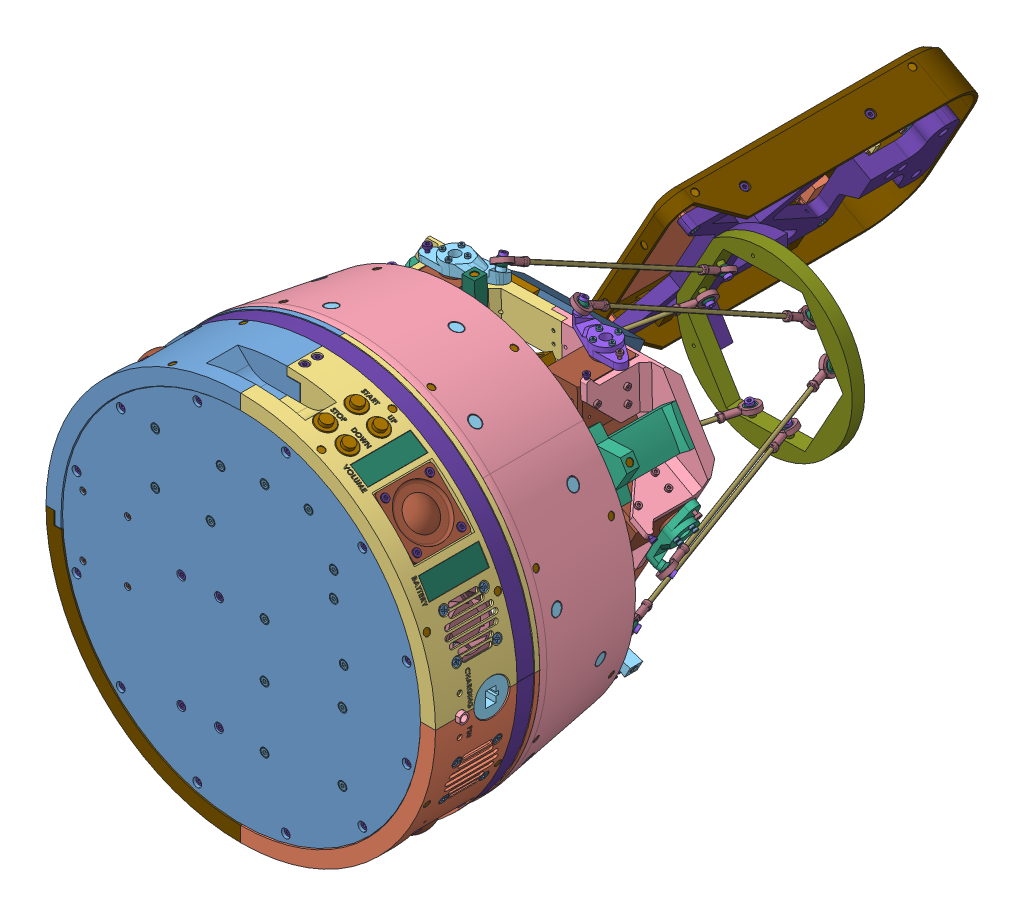
SolidWorks assembly robot xavier, configuration Défaut. Lengths in mm. (continued)
Components (placement in the parent): (continued)
- base-1: base [Défaut] at (-67.3784 29.2661 438.4062) size (438.41 438.41 173) (continued)
  - M3x12mm plastic-7: M3x12mm plastic [Défaut] at (-130.5258 63.5682 511.18) x (-0.383049 0.923728 0) z (0 0 -1) size (5.5 5.5 14.3)
  - M3x12mm plastic-8: M3x12mm plastic [Défaut] at (-130.5258 -42.0524 511.18) x (-0.924031 0.382318 0) z (0 0 -1) size (5.5 5.5 14.3)
  - magnet 5x1.6-2: magnet 5x1.6 [Défaut] at (-144.384 69.3085 585.18) x (-0.146447 -0.353553 0.92388) z (-0.92388 0.382683 0) size (5 5 1.6)
  - magnet 5x1.6-3: magnet 5x1.6 [Défaut] at (-61.581 152.1115 585.18) x (-0.353553 -0.146447 0.92388) z (-0.382683 0.92388 0) size (5 5 1.6)
  - magnet 5x1.6-4: magnet 5x1.6 [Défaut] at (55.5202 152.1115 585.18) x (-0.353553 0.146447 0.92388) z (0.382683 0.92388 0) size (5 5 1.6)
  - magnet 5x1.6-5: magnet 5x1.6 [Défaut] at (138.3232 69.3085 585.18) x (-0.146447 0.353553 0.92388) z (0.92388 0.382683 0) size (5 5 1.6)
  - magnet 5x1.6-6: magnet 5x1.6 [Défaut] at (138.3232 -47.7926 585.18) x (0.146447 0.353553 0.92388) z (0.92388 -0.382683 0) size (5 5 1.6)
  - magnet 5x1.6-7: magnet 5x1.6 [Défaut] at (55.5202 -130.5956 585.18) x (0.353553 0.146447 0.92388) z (0.382683 -0.92388 0) size (5 5 1.6)
  - magnet 5x1.6-8: magnet 5x1.6 [Défaut] at (-61.581 -130.5956 585.18) x (0.353553 -0.146447 0.92388) z (-0.382683 -0.92388 0) size (5 5 1.6)
  - magnet 5x1.6-10: magnet 5x1.6 [Défaut] at (-133.1214 -43.1275 427.3698) x (-0.137009 0.642728 -0.753744) z (-0.912505 -0.377972 -0.156434) size (5 5 1.6)
  - magnet 5x1.6-11: magnet 5x1.6 [Défaut] at (-133.1214 64.6434 427.3698) x (0.357597 0.551357 -0.753744) z (-0.912505 0.377972 -0.156434) size (5 5 1.6)
  - magnet 5x1.6-12: magnet 5x1.6 [Défaut] at (-56.9159 140.849 427.3698) x (0.642728 0.137009 -0.753744) z (-0.377972 0.912505 -0.156434) size (5 5 1.6)
  - magnet 5x1.6-13: magnet 5x1.6 [Défaut] at (50.8551 140.849 427.3698) x (0.551357 -0.357597 -0.753744) z (0.377972 0.912505 -0.156434) size (5 5 1.6)
  - magnet 5x1.6-14: magnet 5x1.6 [Défaut] at (127.0606 64.6434 427.3698) x (0.137009 -0.642728 -0.753744) z (0.912505 0.377972 -0.156434) size (5 5 1.6)
  - magnet 5x1.6-15: magnet 5x1.6 [Défaut] at (127.0606 -43.1275 427.3698) x (-0.357597 -0.551357 -0.753744) z (0.912505 -0.377972 -0.156434) size (5 5 1.6)
  - magnet 5x1.6-16: magnet 5x1.6 [Défaut] at (50.8551 -119.3331 427.3698) x (-0.642728 -0.137009 -0.753744) z (0.377972 -0.912505 -0.156434) size (5 5 1.6)
  - magnet 5x1.6-18: magnet 5x1.6 [Défaut] at (-143.3897 -47.3808 497.5426) x (-0.137009 0.642728 -0.753744) z (-0.912505 -0.377972 -0.156434) size (5 5 1.6)
  - magnet 5x1.6-19: magnet 5x1.6 [Défaut] at (-143.3897 68.8967 497.5426) x (0.357597 0.551357 -0.753744) z (-0.912505 0.377972 -0.156434) size (5 5 1.6)
  - magnet 5x1.6-20: magnet 5x1.6 [Défaut] at (-61.1691 151.1172 497.5426) x (0.642728 0.137009 -0.753744) z (-0.377972 0.912505 -0.156434) size (5 5 1.6)
  - magnet 5x1.6-21: magnet 5x1.6 [Défaut] at (55.1083 151.1172 497.5426) x (0.551357 -0.357597 -0.753744) z (0.377972 0.912505 -0.156434) size (5 5 1.6)
  - magnet 5x1.6-22: magnet 5x1.6 [Défaut] at (137.3289 68.8967 497.5426) x (0.137009 -0.642728 -0.753744) z (0.912505 0.377972 -0.156434) size (5 5 1.6)
  - magnet 5x1.6-23: magnet 5x1.6 [Défaut] at (137.3289 -47.3808 497.5426) x (-0.357597 -0.551357 -0.753744) z (0.912505 -0.377972 -0.156434) size (5 5 1.6)
  - magnet 5x1.6-24: magnet 5x1.6 [Défaut] at (55.1083 -129.6014 497.5426) x (-0.642728 -0.137009 -0.753744) z (0.377972 -0.912505 -0.156434) size (5 5 1.6)
  - magnet 5x1.6-26: magnet 5x1.6 [Défaut] at (-144.384 69.3085 528.68) x (-0.146447 -0.353553 0.92388) z (-0.92388 0.382683 0) size (5 5 1.6)
  - magnet 5x1.6-27: magnet 5x1.6 [Défaut] at (-61.581 152.1115 528.68) x (-0.353553 -0.146447 0.92388) z (-0.382683 0.92388 0) size (5 5 1.6)
  - magnet 5x1.6-28: magnet 5x1.6 [Défaut] at (55.5202 152.1115 528.68) x (-0.353553 0.146447 0.92388) z (0.382683 0.92388 0) size (5 5 1.6)
  - magnet 5x1.6-29: magnet 5x1.6 [Défaut] at (138.3232 69.3085 528.68) x (-0.146447 0.353553 0.92388) z (0.92388 0.382683 0) size (5 5 1.6)
  - magnet 5x1.6-30: magnet 5x1.6 [Défaut] at (138.3232 -47.7926 528.68) x (0.146447 0.353553 0.92388) z (0.92388 -0.382683 0) size (5 5 1.6)
  - magnet 5x1.6-31: magnet 5x1.6 [Défaut] at (55.5202 -130.5956 528.68) x (0.353553 0.146447 0.92388) z (0.382683 -0.92388 0) size (5 5 1.6)
  - magnet 5x1.6-32: magnet 5x1.6 [Défaut] at (-61.581 -130.5956 528.68) x (0.353553 -0.146447 0.92388) z (-0.382683 -0.92388 0) size (5 5 1.6)
- torso bottom xavier-1: torso bottom xavier [Défaut] at (-346.4088 28.5468 798.7391) x (0 0 -1) z (1 0 0) size (138.9 286.86 276.63) (flexible)
  - base gear-1: base gear [Défaut] at (-29.7845 -73.604 101.0471) size (13.91 276 276)
    - base gear 1-1: base gear 1 [Défaut] at (-37.0626 85.0813 174.9529) size (10 121.52 174.95)
    - base gear 2-1: base gear 2 [Défaut] at (-37.0626 85.0813 174.9529) size (10 174.95 121.52)
    - base gear 3-1: base gear 3 [Défaut] at (-37.0626 85.0813 174.9529) size (10 121.52 174.95)
    - base gear 4-1: base gear 4 [Défaut] at (-37.0626 85.0813 174.9529) size (13.91 174.95 121.52)
    - M3x6mm plastic-1: M3x6mm plastic [Défaut] at (-36.0626 58.0825 44.722) x (0 0 -1) z (1 0 0) size (5.5 5.5 8.3)
    - M3x6mm plastic-2: M3x6mm plastic [Défaut] at (-36.0626 215.3121 147.9541) x (0 0 -1) z (1 0 0) size (5.5 5.5 8.3)
    - M3x6mm plastic-3: M3x6mm plastic [Défaut] at (-36.0626 112.08 305.1837) x (0 0 -1) z (1 0 0) size (5.5 5.5 8.3)
    - M3x6mm plastic-4: M3x6mm plastic [Défaut] at (-36.0626 -45.1495 201.9516) x (0 0 -1) z (1 0 0) size (5.5 5.5 8.3)
  - torso bottom external-1: torso bottom external [Défaut] at (174.2366 -65.8734 317.1586) x (0 0.020761 0.999784) z (-1 0 0) size (250 250 10)
    - torso bottom external 1-1: torso bottom external 1 [Défaut] at (-39.5438 78.1885 220.0837) size (220.08 104.52 10)
    - torso bottom external 2-1: torso bottom external 2 [Défaut] at (-39.5438 78.1885 220.0837) size (165.18 170.3 10)
    - torso bottom external 3-1: torso bottom external 3 [Défaut] at (-39.5438 78.1885 220.0837) size (109.03 217.53 10)
    - M3x6mm plastic-1: M3x6mm plastic [Défaut] at (-119.0039 2.1221 229.0837) x (-1 0 0) z (0 0 -1) size (5.5 5.5 8.3)
    - M3x6mm plastic-2: M3x6mm plastic [Défaut] at (-126.2275 -4.793 229.0837) x (-1 0 0) z (0 0 -1) size (5.5 5.5 8.3)
    - M3x6mm plastic-3: M3x6mm plastic [Défaut] at (66.0616 47.4073 229.0837) x (-1 0 0) z (0 0 -1) size (5.5 5.5 8.3)
    - M3x6mm plastic-4: M3x6mm plastic [Défaut] at (75.6621 44.609 229.0837) x (-1 0 0) z (0 0 -1) size (5.5 5.5 8.3)
    - M3x6mm plastic-5: M3x6mm plastic [Défaut] at (-65.6893 185.0362 229.0837) x (-1 0 0) z (0 0 -1) size (5.5 5.5 8.3)
    - M3x6mm plastic-6: M3x6mm plastic [Défaut] at (-68.0662 194.7496 229.0837) x (-1 0 0) z (0 0 -1) size (5.5 5.5 8.3)
  - torso bottom internal xavier-1: torso bottom internal xavier [Défaut] at (-45.8471 11.4773 276) x (0 -0.855458 0.517872) z (-1 0 0) size (168.5 194.56 65)
  - torso bottom holder-1: torso bottom holder [Défaut] at (-69.831 -106.8794 292.5674) x (0 -0.855458 0.517872) z (0 0.517872 0.855458) size (29.5 23 26.69)
    - torso bottom holder-1: torso bottom holder [Défaut] at (-16.159 -8.0161 32.1209) size (29.5 22 26.69)
    - 605zz-1: 605zz [Défaut] at (5.461 -2.0161 24.075) x (0.190809 0 0.981627) z (-0.981627 0 0.190809) size (14 14 5)
    - M5 washer-1: M5 washer [Défaut] at (0.5529 -2.0161 25.029) x (0.190809 0 0.981627) z (-0.981627 0 0.190809) size (10 10 1.1)
    - M5 washer-2: M5 washer [Défaut] at (6.5408 -2.0161 23.8651) x (0.190809 0 0.981627) z (-0.981627 0 0.190809) size (10 10 1.1)
    - M5x16mm socket-1: M5x16mm socket [Défaut] at (10.0747 -2.0161 23.1782) x (-0.981627 0 0.190809) z (-0.132069 -0.72175 -0.679437) size (21 8.5 8.5)
  - torso bottom holder-2: torso bottom holder [Défaut] at (-69.831 85.0034 370.2162) x (0 0.876219 0.481912) z (0 0.481912 -0.876219) size (29.5 23 26.69)
    - torso bottom holder-1: torso bottom holder [Défaut] at (-16.159 -8.0161 32.1209) size (29.5 22 26.69)
    - 605zz-1: 605zz [Défaut] at (5.461 -2.0161 24.075) x (0.190809 0 0.981627) z (-0.981627 0 0.190809) size (14 14 5)
    - M5 washer-1: M5 washer [Défaut] at (0.5529 -2.0161 25.029) x (0.190809 0 0.981627) z (-0.981627 0 0.190809) size (10 10 1.1)
    - M5 washer-2: M5 washer [Défaut] at (6.5408 -2.0161 23.8651) x (0.190809 0 0.981627) z (-0.981627 0 0.190809) size (10 10 1.1)
    - M5x16mm socket-1: M5x16mm socket [Défaut] at (10.0747 -2.0161 23.1782) x (-0.981627 0 0.190809) z (-0.132069 -0.72175 -0.679437) size (21 8.5 8.5)
  - torso bottom holder-3: torso bottom holder [Défaut] at (-69.831 56.3078 165.2164) x (0 -0.020761 -0.999784) z (0 -0.999784 0.020761) size (29.5 23 26.69)
    - torso bottom holder-1: torso bottom holder [Défaut] at (-16.159 -8.0161 32.1209) size (29.5 22 26.69)
    - 605zz-1: 605zz [Défaut] at (5.461 -2.0161 24.075) x (0.190809 0 0.981627) z (-0.981627 0 0.190809) size (14 14 5)
    - M5 washer-1: M5 washer [Défaut] at (0.5529 -2.0161 25.029) x (0.190809 0 0.981627) z (-0.981627 0 0.190809) size (10 10 1.1)
    - M5 washer-2: M5 washer [Défaut] at (6.5408 -2.0161 23.8651) x (0.190809 0 0.981627) z (-0.981627 0 0.190809) size (10 10 1.1)
    - M5x16mm socket-1: M5x16mm socket [Défaut] at (10.0747 -2.0161 23.1782) x (-0.981627 0 0.190809) z (-0.132069 -0.72175 -0.679437) size (21 8.5 8.5)
  - limit switch bracket-1: limit switch bracket [Défaut] at (-45.8471 11.4773 276) x (0 -0.810958 -0.585105) z (1 0 0) size (34.42 36.22 10)
  - stewart stand-1: stewart stand [Défaut] at (-45.8471 11.4773 276) x (0 0.174686 -0.984624) z (1 0 0) size (47.84 42.37 60)
  - stewart stand-2: stewart stand [Défaut] at (-45.8471 11.4773 276) x (0 0.765367 0.643594) z (1 0 0) size (47.84 42.37 60)
  - stewart stand-3: stewart stand [Défaut] at (-45.8471 11.4773 276) x (0 -0.940053 0.34103) z (1 0 0) size (47.84 42.37 60)
  - limit switch-1: limit switch [Défaut] at (-39.8471 -70.7788 381.8891) x (0 0.810958 0.585105) z (0 0.585105 -0.810958) size (20 16.7 6)
  - slip ring (SNM220A-24)-1: slip ring (SNM220A-24) [Défaut] at (-108.3471 11.4773 276) x (0 -0.517872 -0.855458) z (1 0 0) size (44 44 66.3)
  - Jetson AGX Xavier-1: Jetson AGX Xavier [Défaut] at (-61.5471 20.168 283.5975) x (0 -0.855458 0.517872) z (1 0 0) size (105 105 65.46)
  - gear servo bracket-1: gear servo bracket [Défaut] at (-92.1471 -13.8325 196.3361) x (0 0.855458 -0.517872) z (1 0 0) size (80.9 110.9 63)
    - gear servo bracket-1: gear servo bracket [Défaut] at (-19.6043 81.2564 46.3) size (55 84.8 42)
    - XL430-W250-T-1: XL430-W250-T [Défaut] at (-13.6043 10.5064 84.3) x (0 -1 0) z (0 0 -1) size (28.5 46.5 36)
    - torso bottom gear-1: torso bottom gear [Metric - Spur gear 1.5M 52T 20PA 10FW ---S52N75H50L9N] at (-25.6043 10.5064 35.3) x (0 0 -1) z (0 1 0) size (23 80.9 80.9)
    - M2.5x8mm plastic-1: M2.5x8mm plastic [Défaut] at (-21.6043 -0.7436 73.3) x (1 0 0) z (0 -1 0) size (4.5 4.5 9.9)
    - M2.5x8mm plastic-2: M2.5x8mm plastic [Défaut] at (2.3957 -0.7436 73.3) x (1 0 0) z (0 -1 0) size (4.5 4.5 9.9)
    - M2.5x8mm plastic-3: M2.5x8mm plastic [Défaut] at (-21.6043 -0.7436 61.3) x (1 0 0) z (0 -1 0) size (4.5 4.5 9.9)
    - M2.5x8mm plastic-4: M2.5x8mm plastic [Défaut] at (2.3957 -0.7436 61.3) x (1 0 0) z (0 -1 0) size (4.5 4.5 9.9)
    - M2.5x8mm plastic-5: M2.5x8mm plastic [Défaut] at (-34.1043 2.5064 61.3) x (0 0 1) z (-1 0 0) size (4.5 4.5 9.9)
    - M2.5x8mm plastic-6: M2.5x8mm plastic [Défaut] at (-34.1043 18.5064 61.3) x (0 0 1) z (-1 0 0) size (4.5 4.5 9.9)
    - M2x12mm socket-1: M2x12mm socket [Défaut] at (-25.6043 18.5064 51.3) x (-0.923728 -0.383049 0) z (0 0 -1) size (3.8 3.8 13.6)
    - M2x12mm socket-2: M2x12mm socket [Défaut] at (-33.6043 10.5064 51.3) x (1 0 0) z (0 0 -1) size (3.8 3.8 13.6)
    - M2x12mm socket-3: M2x12mm socket [Défaut] at (-17.6043 10.5064 51.3) x (-0.923728 -0.383049 0) z (0 0 -1) size (3.8 3.8 13.6)
    - M2x12mm socket-4: M2x12mm socket [Défaut] at (-25.6043 2.5064 51.3) x (1 0 0) z (0 0 -1) size (3.8 3.8 13.6)
  - torso bottom magnet bracket-1: torso bottom magnet bracket [Défaut] at (-45.8471 11.4773 276) x (0 0.999784 -0.020761) z (1 0 0) size (36.32 10 10)
  - M3x12mm plastic-15: M3x12mm plastic [Défaut] at (-51.8471 81.7797 184.9913) x (0 -0.271233 -0.962514) z (1 0 0) size (5.5 5.5 14.3)
  - M3x12mm plastic-16: M3x12mm plastic [Défaut] at (-51.8471 50.6877 167.8911) x (0 -0.296568 -0.955012) z (1 0 0) size (5.5 5.5 14.3)
  - M3x12mm plastic-17: M3x12mm plastic [Défaut] at (-51.8471 85.4972 364.0117) x (0 -0.296568 -0.955012) z (1 0 0) size (5.5 5.5 14.3)
  - M3x12mm plastic-18: M3x12mm plastic [Défaut] at (-51.8471 55.1419 382.388) x (0 -0.296568 -0.955012) z (1 0 0) size (5.5 5.5 14.3)
  - M3x12mm plastic-19: M3x12mm plastic [Défaut] at (-51.8471 -101.753 296.0973) x (0 -0.296568 -0.955012) z (1 0 0) size (5.5 5.5 14.3)
  - M3x12mm plastic-20: M3x12mm plastic [Défaut] at (-51.8471 -102.4897 260.6207) x (0 -0.296568 -0.955012) z (1 0 0) size (5.5 5.5 14.3)
  - M3x12mm plastic-1: M3x12mm plastic [Défaut] at (-50.8471 -86.7427 325.5236) x (-0.5 0.44849 0.740848) z (0 0.855458 -0.517872) size (5.5 5.5 14.3)
  - M3x12mm plastic-2: M3x12mm plastic [Défaut] at (-50.8471 -77.9389 340.0664) x (-0.5 0.44849 0.740848) z (0 0.855458 -0.517872) size (5.5 5.5 14.3)
  - M3x12mm plastic-3: M3x12mm plastic [Défaut] at (-50.8471 103.476 336.2992) x (-0.5 -0.417348 0.758828) z (0 -0.876219 -0.481912) size (5.5 5.5 14.3)
  - M3x12mm plastic-4: M3x12mm plastic [Défaut] at (-50.8471 111.6685 321.4035) x (-0.5 -0.417348 0.758828) z (0 -0.876219 -0.481912) size (5.5 5.5 14.3)
  - M3x12mm plastic-5: M3x12mm plastic [Défaut] at (-50.8471 17.6986 166.1772) x (1 0 0) z (0 0.020761 0.999784) size (5.5 5.5 14.3)
  - M3x12mm plastic-6: M3x12mm plastic [Défaut] at (-50.8471 0.7022 166.5301) x (1 0 0) z (0 0.020761 0.999784) size (5.5 5.5 14.3)
  - M5x16mm socket-1: M5x16mm socket [Défaut] at (-51.8471 -94.3262 217.8091) x (0 0.876219 0.481912) z (-1 0 0) size (21 8.5 8.5)
  - M5x16mm socket-2: M5x16mm socket [Défaut] at (-51.8471 13.9842 396.724) x (0 -0.020761 -0.999784) z (0.874242 0.485385 -0.010079) size (21 8.5 8.5)
  - M5x16mm socket-3: M5x16mm socket [Défaut] at (-51.8471 114.7739 213.4669) x (0 -0.855458 0.517872) z (-1 0 0) size (21 8.5 8.5)
  - 605zz-1: 605zz [Défaut] at (-51.8471 -87.1193 221.7728) x (-0.5 -0.417348 0.758828) z (0 -0.876219 -0.481912) size (14 14 5)
  - 605zz-2: 605zz [Défaut] at (-51.8471 107.7377 217.7264) x (-0.5 0.44849 0.740848) z (0 0.855458 -0.517872) size (14 14 5)
  - 605zz-3: 605zz [Défaut] at (-51.8471 13.8135 388.5007) x (1 0 0) z (0 0.020761 0.999784) size (14 14 5)
  - M5 washer-1: M5 washer [Défaut] at (-51.8471 -86.1555 222.3029) x (0.785714 -0.298106 0.54202) z (0 -0.876219 -0.481912) size (10 10 1.1)
  - M5 washer-2: M5 washer [Défaut] at (-51.8471 -91.5004 219.3632) x (-0.5 -0.417348 0.758828) z (0 -0.876219 -0.481912) size (10 10 1.1)
  - M5 washer-3: M5 washer [Défaut] at (-51.8471 106.7967 218.2961) x (0.785714 0.32035 0.529177) z (0 0.855458 -0.517872) size (10 10 1.1)
  - M5 washer-4: M5 washer [Défaut] at (-51.8471 112.015 215.1371) x (-0.5 0.44849 0.740848) z (0 0.855458 -0.517872) size (10 10 1.1)
  - M5 washer-5: M5 washer [Défaut] at (-51.8471 13.7906 387.401) x (1 0 0) z (0 0.020761 0.999784) size (10 10 1.1)
  - M5 washer-6: M5 washer [Défaut] at (-51.8471 13.9173 393.4997) x (1 0 0) z (0 0.020761 0.999784) size (10 10 1.1)
  - M5x30mm socket-1: M5x30mm socket [Défaut] at (-51.8471 8.9097 152.3567) x (0 0.020761 0.999784) z (-0.999286 0.037779 -0.000785) size (35 8.5 8.5)
  - M5x30mm socket-2: M5x30mm socket [Défaut] at (-51.8471 119.8393 335.5981) x (0 -0.876219 -0.481912) z (-0.551976 0.401848 -0.730644) size (35 8.5 8.5)
  - M5x30mm socket-3: M5x30mm socket [Défaut] at (-51.8471 -94.3172 340.0452) x (0 0.855458 -0.517872) z (0.446156 0.463472 0.765597) size (35 8.5 8.5)
  - 605zz-4: 605zz [Défaut] at (-51.8471 9.0373 158.5003) x (1 0 0) z (0 0.020761 0.999784) size (14 14 5)
  - 605zz-5: 605zz [Défaut] at (-51.8471 110.0739 330.2272) x (1 0 0) z (0 0.876219 0.481912) size (14 14 5)
  - 605zz-6: 605zz [Défaut] at (-51.8471 -84.7831 334.2736) x (1 0 0) z (0 -0.855458 0.517872) size (14 14 5)
  - M5 washer-7: M5 washer [Défaut] at (-51.8471 9.1411 163.4993) x (1 0 0) z (0 0.020761 0.999784) size (10 10 1.1)
  - M5 washer-8: M5 washer [Défaut] at (-51.8471 9.0145 157.4006) x (1 0 0) z (0 0.020761 0.999784) size (10 10 1.1)
  - M5 washer-9: M5 washer [Défaut] at (-51.8471 114.455 332.6368) x (1 0 0) z (0 0.876219 0.481912) size (10 10 1.1)
  - M5 washer-10: M5 washer [Défaut] at (-51.8471 109.11 329.6971) x (1 0 0) z (0 0.876219 0.481912) size (10 10 1.1)
  - M5 washer-11: M5 washer [Défaut] at (-51.8471 -89.0604 336.8629) x (1 0 0) z (0 -0.855458 0.517872) size (10 10 1.1)
  - M5 washer-12: M5 washer [Défaut] at (-51.8471 -83.8421 333.7039) x (1 0 0) z (0 -0.855458 0.517872) size (10 10 1.1)
  - M3x12mm plastic-7: M3x12mm plastic [Défaut] at (-60.8471 92.7993 333.2803) x (-1 0 0) z (0 0.481912 -0.876219) size (5.5 5.5 14.3)
  - M3x12mm plastic-8: M3x12mm plastic [Défaut] at (-68.6271 92.7993 333.2803) x (-1 0 0) z (0 0.481912 -0.876219) size (5.5 5.5 14.3)
  - M3x12mm plastic-9: M3x12mm plastic [Défaut] at (-60.8471 -78.7899 317.7868) x (1 0 0) z (0 0.517872 0.855458) size (5.5 5.5 14.3)
  - M3x12mm plastic-10: M3x12mm plastic [Défaut] at (-68.6271 -78.7899 317.7868) x (1 0 0) z (0 0.517872 0.855458) size (5.5 5.5 14.3)
  - M3x12mm plastic-11: M3x12mm plastic [Défaut] at (-60.8471 20.4225 176.9329) x (-0.887003 -0.009587 -0.461665) z (0 -0.999784 0.020761) size (5.5 5.5 14.3)
  - M3x12mm plastic-12: M3x12mm plastic [Défaut] at (-68.6271 20.4225 176.9329) x (-1 0 0) z (0 -0.999784 0.020761) size (5.5 5.5 14.3)
  - M3x12mm plastic-13: M3x12mm plastic [Défaut] at (-51.8471 -61.3776 364.9784) x (0 -0.247285 -0.968943) z (1 0 0) size (5.5 5.5 14.3)
  - M3x12mm plastic-14: M3x12mm plastic [Défaut] at (-51.8471 -49.9908 373.194) x (0 -0.231986 -0.972719) z (1 0 0) size (5.5 5.5 14.3)
  - M2.5x12mm plastic-1: M2.5x12mm plastic [Défaut] at (-39.8471 -63.7575 372.1576) x (1 0 0) z (0 -0.585105 0.810958) size (4.5 4.5 13.9)
  - M2.5x12mm plastic-2: M2.5x12mm plastic [Défaut] at (-39.8471 -56.0534 377.7161) x (1 0 0) z (0 -0.585105 0.810958) size (4.5 4.5 13.9)
  - M5x10mm plastic-1: M5x10mm plastic [Défaut] at (-100.7471 20.5401 290.9705) x (0 0.996614 0.082224) z (-1 0 0) size (8.5 8.5 13.5)
  - M5x10mm plastic-2: M5x10mm plastic [Défaut] at (-100.7471 -6.0189 276.3633) x (0 0.996614 0.082224) z (-1 0 0) size (8.5 8.5 13.5)
  - M5x10mm plastic-3: M5x10mm plastic [Défaut] at (-100.7471 19.9108 260.6662) x (0 -0.304563 -0.952492) z (-1 0 0) size (8.5 8.5 13.5)
  - M3x55mm socket-1: M3x55mm socket [Défaut] at (-27.5471 35.6969 220.4243) x (0 -0.689816 -0.723985) z (-1 0 0) size (5.5 5.5 58)
  - M3x55mm socket-2: M3x55mm socket [Défaut] at (-27.5471 -2.0933 335.6497) x (0 -0.811134 -0.58486) z (-1 0 0) size (5.5 5.5 58)
  - M3x55mm socket-3: M3x55mm socket [Défaut] at (-27.5471 -43.0052 268.0685) x (0 -0.689816 -0.723985) z (-1 0 0) size (5.5 5.5 58)
  - M3x55mm socket-4: M3x55mm socket [Défaut] at (-27.5471 76.6088 288.0055) x (0 -0.689816 -0.723985) z (-1 0 0) size (5.5 5.5 58)
  - M3x12mm plastic-21: M3x12mm plastic [Défaut] at (-51.8471 -54.0432 187.0783) x (0 -0.811134 -0.58486) z (1 0 0) size (5.5 5.5 14.3)
  - M3x12mm plastic-22: M3x12mm plastic [Défaut] at (-51.8471 -36.9341 176.7209) x (0 -0.812851 -0.582471) z (1 0 0) size (5.5 5.5 14.3)
  - M3x12mm plastic-23: M3x12mm plastic [Défaut] at (-51.8471 -42.1128 168.1663) x (0 -0.812851 -0.582471) z (1 0 0) size (5.5 5.5 14.3)
  - M3x12mm plastic-24: M3x12mm plastic [Défaut] at (-51.8471 -59.2219 178.5238) x (0 -0.811134 -0.58486) z (1 0 0) size (5.5 5.5 14.3)
  - magnet 5x1.6-7: magnet 5x1.6 [Défaut] at (-40.8471 83.5192 395.004) x (-1 0 0) z (0 0.517872 0.855458) size (5 5 1.6)
  - magnet 5x1.6-12: magnet 5x1.6 [Défaut] at (-40.8471 150.5588 273.1119) x (-1 0 0) z (0 0.999784 -0.020761) size (5 5 1.6)
  - magnet 5x1.6-11: magnet 5x1.6 [Défaut] at (-40.8471 78.5168 154.1078) x (-1 0 0) z (0 0.481912 -0.876219) size (5 5 1.6)
  - magnet 5x1.6-10: magnet 5x1.6 [Défaut] at (-40.8471 -60.5646 156.996) x (-1 0 0) z (0 -0.517872 -0.855458) size (5 5 1.6)
  - magnet 5x1.6-9: magnet 5x1.6 [Défaut] at (-40.8471 -127.6042 278.8881) x (-1 0 0) z (0 -0.999784 0.020761) size (5 5 1.6)
  - magnet 5x1.6-8: magnet 5x1.6 [Défaut] at (-40.8471 -55.5622 397.8922) x (-1 0 0) z (0 -0.481912 0.876219) size (5 5 1.6)
  - M3x12mm plastic-25: M3x12mm plastic [Défaut] at (-51.8471 121.4536 273.7163) x (0 -0.536119 0.844143) z (1 0 0) size (5.5 5.5 14.3)
  - M3x12mm plastic-26: M3x12mm plastic [Défaut] at (-51.8471 131.4514 273.5086) x (0 -0.536119 0.844143) z (1 0 0) size (5.5 5.5 14.3)
- stewart-1: stewart [Défaut] at (-100.6475 26.8239 383.3519) x (-0.481912 -0.876219 0) z (0 0 1) size (270.43 245.67 405.82)
  - stewart bottom-1: stewart bottom [Défaut] at (51.9082 27.1683 257.1781) size (269.04 236.07 88.26) (flexible)
    - stewart bottom 1-1: stewart bottom 1 [Défaut] at (-78.0467 -7.0357 134.0562) size (128.45 156.06 56.5)
    - stewart bottom 2-1: stewart bottom 2 [Défaut] at (-78.0467 -7.0357 134.0562) size (158.11 109.69 56.5)
    - stewart bottom 3-1: stewart bottom 3 [Défaut] at (-78.0467 -7.0357 134.0562) size (141.45 144.8 56.5)
    - XL430-W250-T-1: XL430-W250-T [Défaut] at (3.9424 14.9098 167.3062) x (-0.5 -0.866025 0) z (0.866025 -0.5 0) size (28.5 46.5 36)
    - XL430-W250-T-2: XL430-W250-T [Défaut] at (-18.0467 52.9962 167.3062) x (1 0 0) z (0 1 0) size (28.5 46.5 36)
    - XL430-W250-T-3: XL430-W250-T [Défaut] at (-56.0576 -89.0132 167.3062) x (-0.5 -0.866025 0) z (0.866025 -0.5 0) size (28.5 46.5 36)
    - XL430-W250-T-4: XL430-W250-T [Défaut] at (-100.0359 -89.0132 167.3062) x (-0.5 0.866025 0) z (-0.866025 -0.5 0) size (28.5 46.5 36)
    - XL430-W250-T-5: XL430-W250-T [Défaut] at (-160.0359 14.9098 167.3062) x (-0.5 0.866025 0) z (-0.866025 -0.5 0) size (28.5 46.5 36)
    - XL430-W250-T-6: XL430-W250-T [Défaut] at (-138.0467 52.9962 167.3062) x (1 0 0) z (0 1 0) size (28.5 46.5 36)
    - stewart horn left M3-1: stewart horn left M3 [Défaut] at (-139.8731 -112.0132 155.3062) x (-0.476018 0.824488 -0.305985) z (0.866025 0.5 0) size (57.5 21 11.59)
    - stewart horn left M2.5-4: stewart horn left M2.5 [Défaut] at (-138.0467 98.9962 155.3062) x (0.993445 0 0.114314) z (0 -1 0) size (57.5 21 11.59)
    - stewart horn left M2.5-3: stewart horn left M2.5 [Défaut] at (43.7796 -8.0902 155.3062) x (-0.497766 -0.862156 -0.09443) z (-0.866025 0.5 0) size (57.5 21 11.59)
    - stewart horn right M3-1: stewart horn right M3 [Défaut] at (-16.2204 -112.0132 155.3062) x (0.498739 0.863841 -0.070978) z (-0.866025 0.5 0) size (57.5 21 11.59)
    - stewart horn right M2.5-2: stewart horn right M2.5 [Défaut] at (-18.0467 98.9962 155.3062) x (-0.994742 0 0.102411) z (0 -1 0) size (57.5 21 11.59)
    - stewart horn right M2.5-3: stewart horn right M2.5 [Défaut] at (-199.8731 -8.0902 155.3062) x (0.474882 -0.82252 -0.312965) z (0.866025 0.5 0) size (57.5 21 11.59)
    - USB hub stand-1: USB hub stand [Défaut] at (-132.7404 -70.3674 134.0562) x (-0.866025 -0.5 0) z (0.5 -0.866025 0) size (19 13.3 30)
    - USB hub stand-2: USB hub stand [Défaut] at (-165.7404 -13.2097 134.0562) x (-0.866025 -0.5 0) z (0.5 -0.866025 0) size (19 13.3 30)
    - USB hub stand-3: USB hub stand [Défaut] at (-5.3531 -39.1905 134.0562) x (0.866025 -0.5 0) z (0.5 0.866025 0) size (19 13.3 30)
    - USB hub stand-4: USB hub stand [Défaut] at (-38.3531 -96.3482 134.0562) x (0.866025 -0.5 0) z (0.5 0.866025 0) size (19 13.3 30)
    - Anker USB-c hub (4 ports)-1: Anker USB-c hub (4 ports) [Défaut] at (-123.9019 -60.7196 129.4897) x (-0.5 0.866025 0) z (0.496732 0.286788 -0.819152) size (96 30 21)
    - Anker USB-c hub (4 ports)-2: Anker USB-c hub (4 ports) [Défaut] at (-31.8608 -60.9106 129.2222) x (0.5 0.866025 0) z (-0.496732 0.286788 -0.819152) size (96 30 21)
    - dynamixel control-1: dynamixel control [Défaut] at (-161.0486 20.1008 190.0562) x (-0.5 -0.866025 0) z (0.866025 -0.5 0) size (36 56 13.6)
    - M3x6mm plastic-1: M3x6mm plastic [Défaut] at (-71.5467 71.3295 143.0562) x (-0.72811 0.685461 0) z (0 0 -1) size (5.5 5.5 8.3)
    - M3x6mm plastic-2: M3x6mm plastic [Défaut] at (-71.5467 62.1628 143.0562) x (-1 0 0) z (0 0 -1) size (5.5 5.5 8.3)
    - M3x6mm plastic-3: M3x6mm plastic [Défaut] at (-21.369 -47.2642 143.0562) x (-1 0 0) z (0 0 -1) size (5.5 5.5 8.3)
    - M3x6mm plastic-4: M3x6mm plastic [Défaut] at (-13.4304 -51.8475 143.0562) x (-1 0 0) z (0 0 -1) size (5.5 5.5 8.3)
    - M3x6mm plastic-5: M3x6mm plastic [Défaut] at (-141.2245 -36.0059 143.0562) x (-1 0 0) z (0 0 -1) size (5.5 5.5 8.3)
    - M3x6mm plastic-6: M3x6mm plastic [Défaut] at (-149.1631 -40.5892 143.0562) x (-1 0 0) z (0 0 -1) size (5.5 5.5 8.3)
    - M2.5x8mm plastic-1: M2.5x8mm plastic [Défaut] at (27.861 10.338 146.3062) x (-0.923728 -0.383049 0) z (0 0 -1) size (4.5 4.5 9.9)
    - M2.5x8mm plastic-2: M2.5x8mm plastic [Défaut] at (19.861 -3.5184 146.3062) x (-0.923728 -0.383049 0) z (0 0 -1) size (4.5 4.5 9.9)
    - M2.5x8mm plastic-3: M2.5x8mm plastic [Défaut] at (-10.0467 75.9962 146.3062) x (-1 0 0) z (0 0 -1) size (4.5 4.5 9.9)
    - M2.5x8mm plastic-4: M2.5x8mm plastic [Défaut] at (-26.0467 75.9962 146.3062) x (-1 0 0) z (0 0 -1) size (4.5 4.5 9.9)
    - M2.5x8mm plastic-5: M2.5x8mm plastic [Défaut] at (-130.0467 75.9962 146.3062) x (-1 0 0) z (0 0 -1) size (4.5 4.5 9.9)
    - M2.5x8mm plastic-6: M2.5x8mm plastic [Défaut] at (-146.0467 75.9962 146.3062) x (-1 0 0) z (0 0 -1) size (4.5 4.5 9.9)
    - M2.5x8mm plastic-7: M2.5x8mm plastic [Défaut] at (-183.9545 10.338 146.3062) x (-0.923728 -0.383049 0) z (0 0 -1) size (4.5 4.5 9.9)
    - M2.5x8mm plastic-8: M2.5x8mm plastic [Défaut] at (-175.9545 -3.5184 146.3062) x (-0.923728 -0.383049 0) z (0 0 -1) size (4.5 4.5 9.9)
    - M2.5x8mm plastic-9: M2.5x8mm plastic [Défaut] at (-123.9545 -93.585 146.3062) x (-1 0 0) z (0 0 -1) size (4.5 4.5 9.9)
    - M2.5x8mm plastic-10: M2.5x8mm plastic [Défaut] at (-115.9545 -107.4414 146.3062) x (-1 0 0) z (0 0 -1) size (4.5 4.5 9.9)
    - M2.5x8mm plastic-11: M2.5x8mm plastic [Défaut] at (-40.139 -107.4414 146.3062) x (-1 0 0) z (0 0 -1) size (4.5 4.5 9.9)
    - M2.5x8mm plastic-12: M2.5x8mm plastic [Défaut] at (-32.139 -93.585 146.3062) x (-0.923728 -0.383049 0) z (0 0 -1) size (4.5 4.5 9.9)
    - M2.5x8mm plastic-13: M2.5x8mm plastic [Défaut] at (-42.139 -110.9055 159.3062) x (-0.75 0.433013 -0.5) z (-0.5 -0.866025 0) size (4.5 4.5 9.9)
    - M2.5x8mm plastic-14: M2.5x8mm plastic [Défaut] at (-52.5313 -104.9055 159.3062) x (-0.75 0.433013 -0.5) z (-0.5 -0.866025 0) size (4.5 4.5 9.9)
    - M2.5x8mm plastic-15: M2.5x8mm plastic [Défaut] at (-103.5622 -104.9055 159.3062) x (0.75 0.433013 -0.5) z (0.5 -0.866025 0) size (4.5 4.5 9.9)
    - M2.5x8mm plastic-16: M2.5x8mm plastic [Défaut] at (-113.9545 -110.9055 159.3062) x (0.75 0.433013 -0.5) z (0.5 -0.866025 0) size (4.5 4.5 9.9)
    - M2.5x8mm plastic-17: M2.5x8mm plastic [Défaut] at (17.861 -6.9825 159.3062) x (-0.75 0.433013 -0.5) z (-0.5 -0.866025 0) size (4.5 4.5 9.9)
    - M2.5x8mm plastic-18: M2.5x8mm plastic [Défaut] at (7.4687 -0.9825 159.3062) x (-0.75 0.433013 -0.5) z (-0.5 -0.866025 0) size (4.5 4.5 9.9)
    - M2.5x8mm plastic-19: M2.5x8mm plastic [Défaut] at (-173.9545 -6.9825 159.3062) x (0.75 0.433013 -0.5) z (0.5 -0.866025 0) size (4.5 4.5 9.9)
    - M2.5x8mm plastic-20: M2.5x8mm plastic [Défaut] at (-163.5622 -0.9825 159.3062) x (0.75 0.433013 -0.5) z (0.5 -0.866025 0) size (4.5 4.5 9.9)
    - M2.5x8mm plastic-21: M2.5x8mm plastic [Défaut] at (-126.0467 75.9962 159.3062) x (0 0 1) z (1 0 0) size (4.5 4.5 9.9)
    - M2.5x8mm plastic-22: M2.5x8mm plastic [Défaut] at (-126.0467 63.9962 159.3062) x (0 0 1) z (1 0 0) size (4.5 4.5 9.9)
    - M2.5x8mm plastic-23: M2.5x8mm plastic [Défaut] at (-6.0467 75.9962 159.3062) x (0 0 1) z (1 0 0) size (4.5 4.5 9.9)
    - M2.5x8mm plastic-24: M2.5x8mm plastic [Défaut] at (-6.0467 63.9962 159.3062) x (0 0 1) z (1 0 0) size (4.5 4.5 9.9)
    - M2.5x8mm plastic-25: M2.5x8mm plastic [Défaut] at (19.4687 19.8021 159.3062) x (0.75 -0.433013 -0.5) z (0.5 0.866025 0) size (4.5 4.5 9.9)
    - M2.5x8mm plastic-26: M2.5x8mm plastic [Défaut] at (29.861 13.8021 159.3062) x (0.75 -0.433013 -0.5) z (0.5 0.866025 0) size (4.5 4.5 9.9)
    - M2.5x8mm plastic-27: M2.5x8mm plastic [Défaut] at (-40.5313 -84.1209 159.3062) x (0.75 -0.433013 -0.5) z (0.5 0.866025 0) size (4.5 4.5 9.9)
    - M2.5x8mm plastic-28: M2.5x8mm plastic [Défaut] at (-30.139 -90.1209 159.3062) x (-0.75 0.433013 0.5) z (0.5 0.866025 0) size (4.5 4.5 9.9)
    - M2.5x8mm plastic-29: M2.5x8mm plastic [Défaut] at (-185.9545 13.8021 159.3062) x (-0.75 -0.433013 -0.5) z (-0.5 0.866025 0) size (4.5 4.5 9.9)
    - M2.5x8mm plastic-30: M2.5x8mm plastic [Défaut] at (-175.5622 19.8021 159.3062) x (-0.75 -0.433013 -0.5) z (-0.5 0.866025 0) size (4.5 4.5 9.9)
    - M2.5x8mm plastic-31: M2.5x8mm plastic [Défaut] at (-150.0467 63.9962 159.3062) x (0 0 1) z (-1 0 0) size (4.5 4.5 9.9)
    - M2.5x8mm plastic-32: M2.5x8mm plastic [Défaut] at (-150.0467 75.9962 159.3062) x (0 0 -1) z (-1 0 0) size (4.5 4.5 9.9)
    - M2.5x8mm plastic-33: M2.5x8mm plastic [Défaut] at (-30.0467 75.9962 159.3062) x (0 0 1) z (-1 0 0) size (4.5 4.5 9.9)
    - M2.5x8mm plastic-34: M2.5x8mm plastic [Défaut] at (-30.0467 63.9962 159.3062) x (0 0 1) z (-1 0 0) size (4.5 4.5 9.9)
    - M2.5x8mm plastic-35: M2.5x8mm plastic [Défaut] at (-125.9545 -90.1209 159.3062) x (-0.75 -0.433013 -0.5) z (-0.5 0.866025 0) size (4.5 4.5 9.9)
    - M2.5x8mm plastic-36: M2.5x8mm plastic [Défaut] at (-115.5622 -84.1209 159.3062) x (-0.75 -0.433013 -0.5) z (-0.5 0.866025 0) size (4.5 4.5 9.9)
    - M2x12mm socket-1: M2x12mm socket [Défaut] at (-127.3908 -107.6332 147.6899) x (0.476467 -0.825265 -0.303179) z (-0.866025 -0.5 0) size (3.8 3.8 13.6)
    - M2x12mm socket-2: M2x12mm socket [Défaut] at (-132.4229 -98.9173 152.8583) x (-0.105513 0.182755 -0.97748) z (-0.866025 -0.5 0) size (3.8 3.8 13.6)
    - M2x12mm socket-3: M2x12mm socket [Défaut] at (-129.8387 -103.3933 162.9225) x (-0.105513 0.182755 -0.97748) z (-0.866025 -0.5 0) size (3.8 3.8 13.6)
    - M2x12mm socket-4: M2x12mm socket [Défaut] at (-124.8066 -112.1091 157.7541) x (0.476467 -0.825265 -0.303179) z (-0.866025 -0.5 0) size (3.8 3.8 13.6)
    - M2x12mm socket-5: M2x12mm socket [Défaut] at (-187.3629 -3.7585 162.9043) x (0.295978 -0.512649 -0.80597) z (-0.866025 -0.5 0) size (3.8 3.8 13.6)
    - M2x12mm socket-6: M2x12mm socket [Défaut] at (-184.8157 -8.1703 152.8025) x (-0.372959 0.645984 -0.666038) z (-0.866025 -0.5 0) size (3.8 3.8 13.6)
    - M2x12mm socket-7: M2x12mm socket [Défaut] at (-189.8666 0.5781 147.7081) x (0.295978 -0.512649 -0.80597) z (-0.866025 -0.5 0) size (3.8 3.8 13.6)
    - M2x12mm socket-8: M2x12mm socket [Défaut] at (-192.4138 4.99 157.8099) x (-0.372959 0.645984 -0.666038) z (-0.866025 -0.5 0) size (3.8 3.8 13.6)
    - M2x12mm socket-9: M2x12mm socket [Défaut] at (-138.9613 85.9962 163.2538) x (-0.769158 0 -0.639059) z (0 1 0) size (3.8 3.8 13.6)
    - M2x12mm socket-10: M2x12mm socket [Défaut] at (-137.1322 85.9962 147.3587) x (-0.769158 0 -0.639059) z (0 1 0) size (3.8 3.8 13.6)
    - M2x12mm socket-11: M2x12mm socket [Défaut] at (-130.0992 85.9962 156.2207) x (-0.769158 0 -0.639059) z (0 1 0) size (3.8 3.8 13.6)
    - M2x12mm socket-12: M2x12mm socket [Défaut] at (-145.9943 85.9962 154.3917) x (-0.769158 0 -0.639059) z (0 1 0) size (3.8 3.8 13.6)
    - M2x12mm socket-13: M2x12mm socket [Défaut] at (-26.0047 85.9962 156.1255) x (0.994742 0 -0.102411) z (0 1 0) size (3.8 3.8 13.6)
    - M2x12mm socket-14: M2x12mm socket [Défaut] at (-18.866 85.9962 147.3483) x (-0.888781 0 -0.458333) z (0 1 0) size (3.8 3.8 13.6)
    - M2x12mm socket-15: M2x12mm socket [Défaut] at (-10.0888 85.9962 154.4869) x (-0.888781 0 -0.458333) z (0 1 0) size (3.8 3.8 13.6)
    - M2x12mm socket-16: M2x12mm socket [Défaut] at (-17.2275 85.9962 163.2642) x (-0.888781 0 -0.458333) z (0 1 0) size (3.8 3.8 13.6)
    - M2x12mm socket-17: M2x12mm socket [Défaut] at (-27.1948 -105.0215 163.286) x (-0.47988 -0.831176 0.280822) z (0.866025 -0.5 0) size (3.8 3.8 13.6)
    - M2x12mm socket-18: M2x12mm socket [Défaut] at (-27.7626 -106.005 147.3264) x (-0.47988 -0.831176 0.280822) z (0.866025 -0.5 0) size (3.8 3.8 13.6)
    - M2x12mm socket-19: M2x12mm socket [Défaut] at (-31.4686 -112.424 155.874) x (-0.47988 -0.831176 0.280822) z (0.866025 -0.5 0) size (3.8 3.8 13.6)
    - M2x12mm socket-20: M2x12mm socket [Défaut] at (-23.4888 -98.6025 154.7384) x (-0.47988 -0.831176 0.280822) z (0.866025 -0.5 0) size (3.8 3.8 13.6)
    - M2x12mm socket-21: M2x12mm socket [Défaut] at (32.1435 -2.2444 163.2705) x (-0.496461 -0.859896 0.118761) z (0.866025 -0.5 0) size (3.8 3.8 13.6)
    - M2x12mm socket-22: M2x12mm socket [Défaut] at (32.899 -0.936 147.342) x (-0.496461 -0.859896 0.118761) z (0.866025 -0.5 0) size (3.8 3.8 13.6)
    - M2x12mm socket-23: M2x12mm socket [Défaut] at (28.5391 -8.4874 154.5508) x (-0.496461 -0.859896 0.118761) z (0.866025 -0.5 0) size (3.8 3.8 13.6)
    - M2x12mm socket-24: M2x12mm socket [Défaut] at (36.5034 5.3071 156.0617) x (-0.488636 -0.846342 0.211992) z (0.866025 -0.5 0) size (3.8 3.8 13.6)
    - M3x12mm plastic-1: M3x12mm plastic [Défaut] at (-0.5983 -15.9549 141.0562) x (-0.923728 -0.383049 0) z (0 0 -1) size (5.5 5.5 14.3)
    - M3x12mm plastic-2: M3x12mm plastic [Défaut] at (-8.0983 -28.9453 141.0562) x (-0.923728 -0.383049 0) z (0 0 -1) size (5.5 5.5 14.3)
    - M3x12mm plastic-3: M3x12mm plastic [Défaut] at (-33.5983 -73.1126 141.0562) x (-1 0 0) z (0 0 -1) size (5.5 5.5 14.3)
    - M3x12mm plastic-4: M3x12mm plastic [Défaut] at (-41.0983 -86.103 141.0562) x (-1 0 0) z (0 0 -1) size (5.5 5.5 14.3)
    - M3x12mm plastic-5: M3x12mm plastic [Défaut] at (-114.9952 -86.103 141.0562) x (-0.923728 -0.383049 0) z (0 0 -1) size (5.5 5.5 14.3)
    - M3x12mm plastic-6: M3x12mm plastic [Défaut] at (-122.4952 -73.1126 141.0562) x (-0.923728 -0.383049 0) z (0 0 -1) size (5.5 5.5 14.3)
    - M3x12mm plastic-7: M3x12mm plastic [Défaut] at (-147.9952 -28.9453 141.0562) x (-0.923728 -0.383049 0) z (0 0 -1) size (5.5 5.5 14.3)
    - M3x12mm plastic-8: M3x12mm plastic [Défaut] at (-155.4952 -15.9549 141.0562) x (-1 0 0) z (0 0 -1) size (5.5 5.5 14.3)
    - M2.5x8mm plastic-37: M2.5x8mm plastic [Défaut] at (-113.9545 -110.9055 183.3062) x (0.75 0.433013 -0.5) z (0.5 -0.866025 0) size (4.5 4.5 9.9)
    - M2.5x8mm plastic-38: M2.5x8mm plastic [Défaut] at (-42.139 -110.9055 183.3062) x (0.75 -0.433013 0.5) z (-0.5 -0.866025 0) size (4.5 4.5 9.9)
    - M3x12mm plastic-9: M3x12mm plastic [Défaut] at (-37.9608 -119.6687 188.0562) x (0.25 0.433013 -0.866025) z (0.866025 -0.5 0) size (5.5 5.5 14.3)
    - M3x12mm plastic-10: M3x12mm plastic [Défaut] at (-118.1327 -119.6687 188.0562) x (0.25 -0.433013 0.866025) z (-0.866025 -0.5 0) size (5.5 5.5 14.3)
    - M3x8mm plastic-6: M3x8mm plastic [Défaut] at (-33.6086 -122.1305 156.5483) x (-0.208097 -0.360435 0.909276) z (0.866025 -0.5 0) size (5.5 5.5 10.3)
    - M2.5x8mm plastic-39: M2.5x8mm plastic [Défaut] at (29.861 13.8021 183.3062) x (0.75 -0.433013 -0.5) z (0.5 0.866025 0) size (4.5 4.5 9.9)
    - M2.5x8mm plastic-40: M2.5x8mm plastic [Défaut] at (-6.0467 75.9962 183.3062) x (0 0 -1) z (1 0 0) size (4.5 4.5 9.9)
    - M2.5x8mm plastic-41: M2.5x8mm plastic [Défaut] at (-185.9545 13.8021 183.3062) x (0.75 0.433013 0.5) z (-0.5 0.866025 0) size (4.5 4.5 9.9)
    - M2.5x8mm plastic-42: M2.5x8mm plastic [Défaut] at (-150.0467 75.9962 183.3062) x (0 0 1) z (-1 0 0) size (4.5 4.5 9.9)
    - M3x8mm plastic-7: M3x8mm plastic [Défaut] at (-122.8825 -121.4418 160.661) x (0.448793 -0.777332 -0.440841) z (-0.866025 -0.5 0) size (5.5 5.5 10.3)
    - M2.5x12mm plastic-1: M2.5x12mm plastic [Défaut] at (-195.6327 14.5653 188.0562) x (0.25 -0.433013 0.866025) z (-0.866025 -0.5 0) size (4.5 4.5 13.9)
    - M2.5x12mm plastic-2: M2.5x12mm plastic [Défaut] at (-155.5467 83.9962 188.0562) x (1 0 0) z (0 1 0) size (4.5 4.5 13.9)
    - M2.5x12mm plastic-3: M2.5x12mm plastic [Défaut] at (-0.5467 83.9962 188.0562) x (1 0 0) z (0 1 0) size (4.5 4.5 13.9)
    - M2.5x12mm plastic-4: M2.5x12mm plastic [Défaut] at (39.5392 14.5653 188.0562) x (0.25 0.433013 -0.866025) z (0.866025 -0.5 0) size (4.5 4.5 13.9)
    - M2.5x8mm plastic-43: M2.5x8mm plastic [Défaut] at (-199.5233 11.3039 160.7831) x (0.356409 -0.617318 -0.701349) z (-0.866025 -0.5 0) size (4.5 4.5 9.9)
